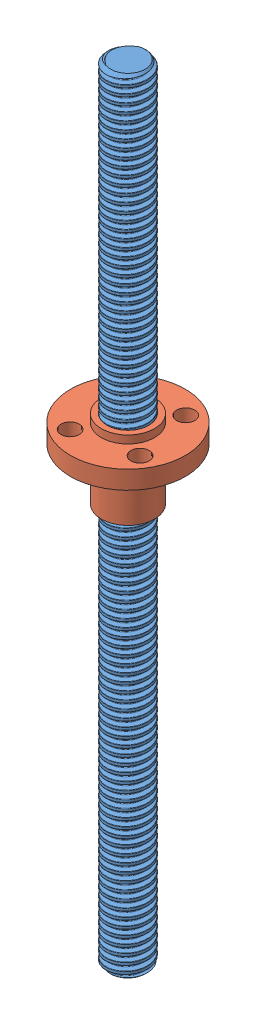
SolidWorks assembly T8LeadScrew, configuration Default. Lengths in mm.
Overall size (30.45 116.78 30.45).
2 component instances, 2 part files, 2 mates.
Components (placement in the parent):
- 8mm trapez mil-1: 8mm trapez mil [Varsayılan] at origin size (8.11 116.78 9.24)
- T8 nut-1: T8 nut [Default] at (0 86.3108 0) x (-0.837169 0 -0.546944) z (0 1 0) size (22 22 15)
Mates (geometry in assembly coordinates):
- Coincident2: coordinate: point of 8mm trapez mil-1
- Concentric1: concentric aligned: cylinder of 8mm trapez mil-1 through (0 115 0) axis (0 -1 0) radius 4; cylinder of T8 nut-1 through (0 89.8108 0) axis (0 -1 0) radius 4
